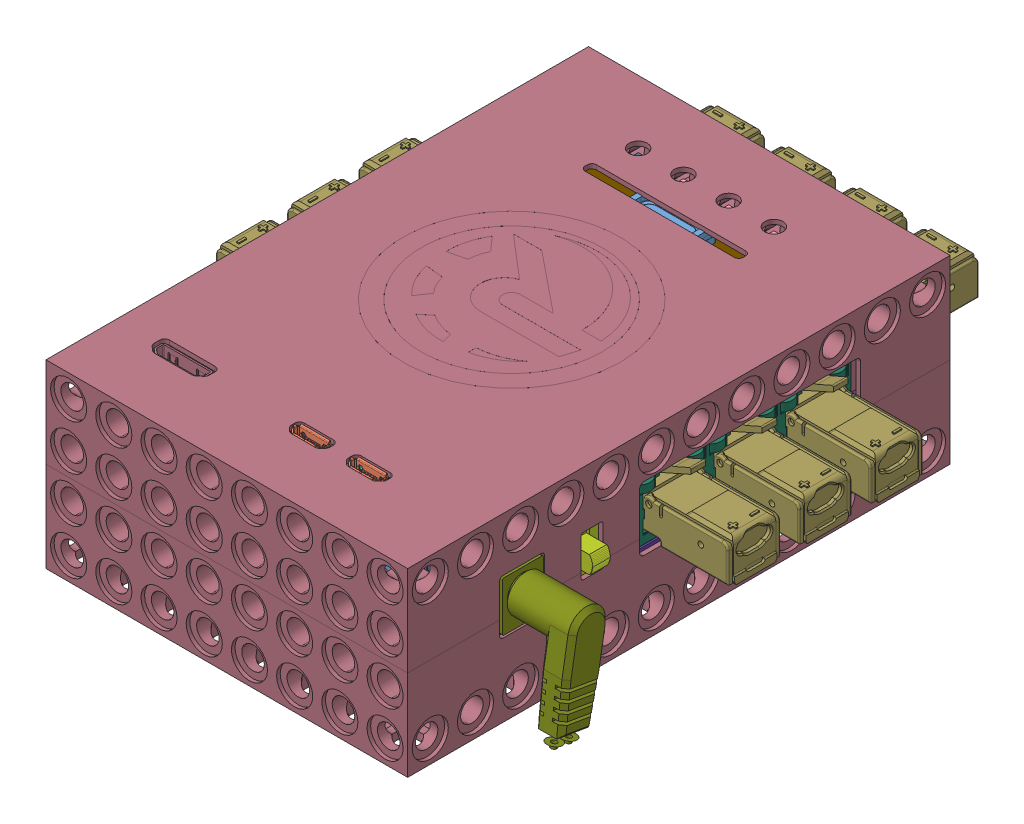
SolidWorks assembly PCBA_estimation_20190215, configuration Default. Lengths in mm. (continued)
Components (placement in the parent): (continued)
- RRRC_carrier_board-1: RRRC_carrier_board [Default] at (75.1836 8.28 47.3515) x (0 0 -1) z (0 1 0) size (102.74 81.4 21.81) (continued)
  - C112_CARRIER_3-1: C112_CARRIER_3 [Default] at origin size (0.5 1 0.5)
    - C_0402_3-1: C_0402_3 [Default] at (82 51.85 0) x (0 1 0) z (0 0 1) size (1 0.5 0.5)
  - D27_CARRIER_3-1: D27_CARRIER_3 [Default] at origin size (1.05 0.65 0.44)
    - SOD-923_3-1: SOD-923_3 [Default] at (80.75 59.9 0) x (1 0 0) z (0 -1 0) size (1.05 0.44 0.65)
  - D28_CARRIER_3-1: D28_CARRIER_3 [Default] at origin size (0.65 1.05 0.44)
    - SOD-923_3-1: SOD-923_3 [Default] at (82.05 55.6 0) x (0 1 0) z (1 0 0) size (1.05 0.44 0.65)
  - FB7_CARRIER_3-1: FB7_CARRIER_3 [Default] at origin size (0.5 1 0.5)
    - IND_0402_3-1: IND_0402_3 [Default] at (80.975 55.775 0) x (0 -1 0) z (0 0 1) size (1 0.5 0.5)
  - FB16_CARRIER_3-1: FB16_CARRIER_3 [Default] at origin size (0.5 1 0.5)
    - IND_0402_3-1: IND_0402_3 [Default] at (81 58.4 0) x (0 -1 0) z (0 0 1) size (1 0.5 0.5)
  - FU19_CARRIER_3-1: FU19_CARRIER_3 [Default] at origin size (2.3 1.5 1.25)
    - BELFUSE_0ZCK_3-1: BELFUSE_0ZCK_3 [Default] at (83.35 57.55 0) x (-1 0 0) z (0 1 0) size (2.3 1.25 1.5)
  - FU20_CARRIER_3-1: FU20_CARRIER_3 [Default] at origin size (2.3 1.5 1.25)
    - BELFUSE_0ZCK_3-1: BELFUSE_0ZCK_3 [Default] at (83.35 59.35 0) x (-1 0 0) z (0 1 0) size (2.3 1.25 1.5)
  - R100_CARRIER_3-1: R100_CARRIER_3 [Default] at origin size (1.15 0.55 0.41)
    - R_0402_3-1: R_0402_3 [Default] at (84.05 55.125 0) x (-1 0 0) z (0 1 0) size (1.15 0.41 0.55)
  - R101_CARRIER_3-1: R101_CARRIER_3 [Default] at origin size (1.15 0.55 0.41)
    - R_0402_3-1: R_0402_3 [Default] at (84.0501 54.1 0) x (-1 0 0) z (0 1 0) size (1.15 0.41 0.55)
  - R104_CARRIER_3-1: R104_CARRIER_3 [Default] at origin size (1.15 0.55 0.41)
    - R_0402_3-1: R_0402_3 [Default] at (84.0501 50.925 0) x (-1 0 0) z (0 1 0) size (1.15 0.41 0.55)
  - R141_CARRIER_3-1: R141_CARRIER_3 [Default] at origin size (1.15 0.55 0.41)
    - R_0402_3-1: R_0402_3 [Default] at (84.0501 56.125 0) x (-1 0 0) z (0 1 0) size (1.15 0.41 0.55)
  - R145_CARRIER_3-1: R145_CARRIER_3 [Default] at origin size (1.15 0.55 0.41)
    - R_0402_3-1: R_0402_3 [Default] at (84.05 52 0) x (1 0 0) z (0 -1 0) size (1.15 0.41 0.55)
  - R146_CARRIER_3-1: R146_CARRIER_3 [Default] at origin size (0.55 1.15 0.41)
    - R_0402_3-1: R_0402_3 [Default] at (81 51.85 0) x (0 1 0) z (1 0 0) size (1.15 0.41 0.55)
  - D21_CARRIER_3-1: D21_CARRIER_3 [Default] at origin size (1.05 0.65 0.44)
    - SOD-923_3-1: SOD-923_3 [Default] at (81.5 39.8 0) x (1 0 0) z (0 -1 0) size (1.05 0.44 0.65)
  - R122_CARRIER_3-1: R122_CARRIER_3 [Default] at origin size (0.55 1.15 0.41)
    - R_0402_3-1: R_0402_3 [Default] at (80.8 41.4 0) x (0 1 0) z (1 0 0) size (1.15 0.41 0.55)
  - R121_CARRIER_3-1: R121_CARRIER_3 [Default] at origin size (1.15 0.55 0.41)
    - R_0402_3-1: R_0402_3 [Default] at (84.05 41.775 0) x (1 0 0) z (0 -1 0) size (1.15 0.41 0.55)
  - R89_CARRIER_3-1: R89_CARRIER_3 [Default] at origin size (1.15 0.55 0.41)
    - R_0402_3-1: R_0402_3 [Default] at (84.05 40.725 0) x (-1 0 0) z (0 1 0) size (1.15 0.41 0.55)
  - R86_CARRIER_3-1: R86_CARRIER_3 [Default] at origin size (1.15 0.55 0.41)
    - R_0402_3-1: R_0402_3 [Default] at (84.05 42.825 0) x (-1 0 0) z (0 1 0) size (1.15 0.41 0.55)
  - R85_CARRIER_3-1: R85_CARRIER_3 [Default] at origin size (1.15 0.55 0.41)
    - R_0402_3-1: R_0402_3 [Default] at (84.05 43.825 0) x (-1 0 0) z (0 1 0) size (1.15 0.41 0.55)
  - R118_CARRIER_3-1: R118_CARRIER_3 [Default] at origin size (1.15 0.55 0.41)
    - R_0402_3-1: R_0402_3 [Default] at (84.05 44.825 0) x (-1 0 0) z (0 1 0) size (1.15 0.41 0.55)
  - FU14_CARRIER_3-1: FU14_CARRIER_3 [Default] at origin size (2.3 1.5 1.25)
    - BELFUSE_0ZCK_3-1: BELFUSE_0ZCK_3 [Default] at (83.3251 48.35 0) x (-1 0 0) z (0 1 0) size (2.3 1.25 1.5)
  - FU13_CARRIER_3-1: FU13_CARRIER_3 [Default] at origin size (2.3 1.5 1.25)
    - BELFUSE_0ZCK_3-1: BELFUSE_0ZCK_3 [Default] at (83.3251 46.5 0) x (-1 0 0) z (0 1 0) size (2.3 1.25 1.5)
  - FB10_CARRIER_3-1: FB10_CARRIER_3 [Default] at origin size (0.5 1 0.5)
    - IND_0402_3-1: IND_0402_3 [Default] at (81.025 48.475 0) x (0 1 0) z (0 0 1) size (1 0.5 0.5)
  - FB4_CARRIER_3-1: FB4_CARRIER_3 [Default] at origin size (0.5 1 0.5)
    - IND_0402_3-1: IND_0402_3 [Default] at (81 45.95 0) x (0 -1 0) z (0 0 1) size (1 0.5 0.5)
  - D19_CARRIER_3-1: D19_CARRIER_3 [Default] at origin size (0.65 1.05 0.44)
    - SOD-923_3-1: SOD-923_3 [Default] at (82 44.55 0) x (0 1 0) z (1 0 0) size (1.05 0.44 0.65)
  - D18_CARRIER_3-1: D18_CARRIER_3 [Default] at origin size (1.05 0.65 0.44)
    - SOD-923_3-1: SOD-923_3 [Default] at (81.5 50 0) x (1 0 0) z (0 -1 0) size (1.05 0.44 0.65)
  - D17_CARRIER_3-1: D17_CARRIER_3 [Default] at origin size (2 2.5 0.6)
    - 6373436816-1: 6373436816 [Default] at (76.7 41.85 0) size (2 2.5 0.6)
      - Extruded_3-1: Extruded_3 [Default] at origin size (2 2.5 0.6)
  - C101_CARRIER_3-1: C101_CARRIER_3 [Default] at origin size (0.5 1 0.5)
    - C_0402_3-1: C_0402_3 [Default] at (81.85 41.4 0) x (0 1 0) z (0 0 1) size (1 0.5 0.5)
  - C99_CARRIER_3-1: C99_CARRIER_3 [Default] at origin size (1.6 3.2 1.6)
    - C_1206_3-1: C_1206_3 [Default] at (78.35 48.05 0) x (0 1 0) z (0 0 1) size (3.2 1.6 1.6)
  - C100_CARRIER_3-1: C100_CARRIER_3 [Default] at origin size (1.6 3.2 1.6)
    - C_1206_3-1: C_1206_3 [Default] at (76.15 46.7 0) x (0 -1 0) z (0 0 1) size (3.2 1.6 1.6)
  - C72_CARRIER_3-1: C72_CARRIER_3 [Default] at origin size (0.5 1 0.5)
    - C_0402_3-1: C_0402_3 [Default] at (79.95 45.95 0) x (0 -1 0) z (0 0 1) size (1 0.5 0.5)
  - C70_CARRIER_3-1: C70_CARRIER_3 [Default] at origin size (0.5 1 0.5)
    - C_0402_3-1: C_0402_3 [Default] at (79.975 48.475 0) x (0 1 0) z (0 0 1) size (1 0.5 0.5)
  - C74_CARRIER_3-1: C74_CARRIER_3 [Default] at origin size (0.5 1 0.5)
    - C_0402_3-1: C_0402_3 [Default] at (79.95 38.3 0) x (0 1 0) z (0 0 1) size (1 0.5 0.5)
  - C76_CARRIER_3-1: C76_CARRIER_3 [Default] at origin size (0.5 1 0.5)
    - C_0402_3-1: C_0402_3 [Default] at (79.975 35.8 0) x (0 -1 0) z (0 0 1) size (1 0.5 0.5)
  - C102_CARRIER_3-1: C102_CARRIER_3 [Default] at origin size (3.2 1.6 1.6)
    - C_1206_3-1: C_1206_3 [Default] at (76.9 38.2 0) x (1 0 0) z (0 0 1) size (3.2 1.6 1.6)
  - C103_CARRIER_3-1: C103_CARRIER_3 [Default] at origin size (3.2 1.6 1.6)
    - C_1206_3-1: C_1206_3 [Default] at (76.9 35.9 0) x (1 0 0) z (0 0 1) size (3.2 1.6 1.6)
  - C105_CARRIER_3-1: C105_CARRIER_3 [Default] at origin size (0.5 1 0.5)
    - C_0402_3-1: C_0402_3 [Default] at (80.9 30.275 0) x (0 1 0) z (0 0 1) size (1 0.5 0.5)
  - D20_CARRIER_3-1: D20_CARRIER_3 [Default] at origin size (2 2.5 0.6)
    - 6373436816-1-1: 6373436816-1 [Default] at (80.7 19.55 0) size (2 2.5 0.6)
      - Extruded_3-1: Extruded_3 [Default] at origin size (2 2.5 0.6)
  - D22_CARRIER_3-1: D22_CARRIER_3 [Default] at origin size (1.05 0.65 0.44)
    - SOD-923_3-1: SOD-923_3 [Default] at (81.4 34 0) x (1 0 0) z (0 -1 0) size (1.05 0.44 0.65)
  - FB5_CARRIER_3-1: FB5_CARRIER_3 [Default] at origin size (0.5 1 0.5)
    - IND_0402_3-1: IND_0402_3 [Default] at (81.025 35.8 0) x (0 -1 0) z (0 0 1) size (1 0.5 0.5)
  - FB12_CARRIER_3-1: FB12_CARRIER_3 [Default] at origin size (0.5 1 0.5)
    - IND_0402_3-1: IND_0402_3 [Default] at (81 38.3 0) x (0 1 0) z (0 0 1) size (1 0.5 0.5)
  - FU15_CARRIER_3-1: FU15_CARRIER_3 [Default] at origin size (2.3 1.5 1.25)
    - BELFUSE_0ZCK_3-1: BELFUSE_0ZCK_3 [Default] at (83.35 35.4 0) x (-1 0 0) z (0 1 0) size (2.3 1.25 1.5)
  - FU16_CARRIER_3-1: FU16_CARRIER_3 [Default] at origin size (2.3 1.5 1.25)
    - BELFUSE_0ZCK_3-1: BELFUSE_0ZCK_3 [Default] at (83.325 38.225 0) x (-1 0 0) z (0 1 0) size (2.3 1.25 1.5)
  - R90_CARRIER_3-1: R90_CARRIER_3 [Default] at origin size (1.15 0.55 0.41)
    - R_0402_3-1: R_0402_3 [Default] at (84.075 32.875 0) x (-1 0 0) z (0 1 0) size (1.15 0.41 0.55)
  - R91_CARRIER_3-1: R91_CARRIER_3 [Default] at origin size (1.15 0.55 0.41)
    - R_0402_3-1: R_0402_3 [Default] at (84.075 31.875 0) x (-1 0 0) z (0 1 0) size (1.15 0.41 0.55)
  - R93_CARRIER_3-1: R93_CARRIER_3 [Default] at origin size (1.15 0.55 0.41)
    - R_0402_3-1: R_0402_3 [Default] at (84.075 33.875 0) x (-1 0 0) z (0 1 0) size (1.15 0.41 0.55)
  - R94_CARRIER_3-1: R94_CARRIER_3 [Default] at origin size (1.15 0.55 0.41)
    - R_0402_3-1: R_0402_3 [Default] at (84.075 29.775 0) x (-1 0 0) z (0 1 0) size (1.15 0.41 0.55)
  - R130_CARRIER_3-1: R130_CARRIER_3 [Default] at origin size (1.15 0.55 0.41)
    - R_0402_3-1: R_0402_3 [Default] at (84.075 30.825 0) x (1 0 0) z (0 -1 0) size (1.15 0.41 0.55)
  - R131_CARRIER_3-1: R131_CARRIER_3 [Default] at origin size (0.55 1.15 0.41)
    - R_0402_3-1: R_0402_3 [Default] at (81.9 30.275 0) x (0 1 0) z (1 0 0) size (1.15 0.41 0.55)
  - CON2_CARRIER_3-1: CON2_CARRIER_3 [Default] at origin size (51.17 16.61 18.92)
    - FCI_RJHSE538103-REVT1_3-1: FCI_RJHSE538103-REVT1_3 [Default] at (75.5745 0.201 0.65) x (1 0 0) z (0 -1 0) size (51.17 18.92 16.61)
  - Y1_CARRIER_3-1: Y1_CARRIER_3 [Default] at origin size (1.5 3.2 0.85)
    - TXC_9HT10_3-1: TXC_9HT10_3 [Default] at (5.75 65.75 0) x (0 -1 0) z (0 0 1) size (3.2 1.5 0.85)
  - U30_CARRIER_3-1: U30_CARRIER_3 [Default] at origin size (6.04 4.9 1.7)
    - SOIC8P127_490X604X170L60X40N_3-1: SOIC8P127_490X604X170L60X40N_3 [Default] at (27.6 30.6 0) x (1 0 0) z (0 0 1) size (6.04 4.9 1.7)
  - U29_CARRIER_3-1: U29_CARRIER_3 [Default] at origin size (14 16 2)
    - Fanstel_BT832A_3-1: Fanstel_BT832A_3 [Default] at (22.05 69 0.3) x (1 0 0) z (0 -1 0) size (14 2 16)
  - U13_CARRIER_3-1: U13_CARRIER_3 [Default] at origin size (3.1 3 0.8)
    - DFN-6(3x3)_0.45_0.95_3x3x1_HD[2,50x1,75]_3-1: DFN-6(3x3)_0.45_0.95_3x3x1_HD[2,50x1,75]_3 [Default] at (59.35 51.35 0.05) x (-1 0 0) z (0 0 1) size (3.1 3 0.8)
  - U27_CARRIER_3-1: U27_CARRIER_3 [Default] at origin size (2.03 2.13 0.6)
    - SON9P50_202X202X60L35X25T130X70_3-1: SON9P50_202X202X60L35X25T130X70_3 [Default] at (7.1 33.1 0) x (0 1 0) z (0 0 1) size (2.13 2.02 0.6)
  - U12_CARRIER_3-1: U12_CARRIER_3 [Default] at origin size (3.1 3 0.8)
    - DFN-6(3x3)_0.45_0.95_3x3x1_HD[2,50x1,75]_3-1: DFN-6(3x3)_0.45_0.95_3x3x1_HD[2,50x1,75]_3 [Default] at (54.25 51.35 0.05) x (1 0 0) z (0 0 1) size (3.1 3 0.8)
  - U25_CARRIER_3-1: U25_CARRIER_3 [Default] at origin size (4.9 6.04 1.7)
    - SOIC8P127_490X604X170L60X40N_3-1: SOIC8P127_490X604X170L60X40N_3 [Default] at (4.5 48.6 0) x (0 1 0) z (0 0 1) size (6.04 4.9 1.7)
  - U11_CARRIER_3-1: U11_CARRIER_3 [Default] at origin size (3.1 3 0.8)
    - DFN-6(3x3)_0.45_0.95_3x3x1_HD[2,50x1,75]_3-1: DFN-6(3x3)_0.45_0.95_3x3x1_HD[2,50x1,75]_3 [Default] at (46.2 51.35 0.05) x (1 0 0) z (0 0 1) size (3.1 3 0.8)
  - U10_CARRIER_3-1: U10_CARRIER_3 [Default] at origin size (4.9 6 1.5)
    - SOIC9P127_490X600X150L72X40T335X271N_3-1: SOIC9P127_490X600X150L72X40T335X271N_3 [Default] at (33.525 23.15 0) x (0 1 0) z (0 0 1) size (6 4.9 1.5)
  - U20_CARRIER_3-1: U20_CARRIER_3 [Default] at origin size (2.03 2.13 0.6)
    - SON9P50_202X202X60L35X25T130X70_3-1: SON9P50_202X202X60L35X25T130X70_3 [Default] at (7.025 58.325 0) x (0 1 0) z (0 0 1) size (2.13 2.02 0.6)
  - U18_CARRIER_3-1: U18_CARRIER_3 [Default] at origin size (3 4.9 1.1)
    - SOP10P50_300X490X110L55X22N_3-1: SOP10P50_300X490X110L55X22N_3 [Default] at (2.65 21.6 0) x (0 -1 0) z (0 0 1) size (4.9 3 1.1)
  - U3_CARRIER_3-1: U3_CARRIER_3 [Default] at origin size (3 3.1 0.8)
    - DFN-6(3x3)_0.45_0.95_3x3x1_HD[2,50x1,75]_3-1: DFN-6(3x3)_0.45_0.95_3x3x1_HD[2,50x1,75]_3 [Default] at (73.15 28.7 0.05) x (0 1 0) z (0 0 1) size (3.1 3 0.8)
  - U14_CARRIER_3-1: U14_CARRIER_3 [Default] at origin size (7.8 7.6 1.6)
    - TSSOP-24[12-12]_0.45_0.65_5.6x7.8x1.6_3-1: TSSOP-24[12-12]_0.45_0.65_5.6x7.8x1.6_3 [Default] at (65.4999 30.5001 0) x (1 0 0) z (0 0 1) size (7.8 7.6 1.6)
  - U9_CARRIER_3-1: U9_CARRIER_3 [Default] at origin size (1.8 2.1 0.5)
    - QFN12P40_170X200X50L50X20N_3-1: QFN12P40_170X200X50L50X20N_3 [Default] at (70.9 51.05 0) size (1.8 2.1 0.5)
  - U8_CARRIER_3-1: U8_CARRIER_3 [Default] at origin size (1.8 2.1 0.5)
    - QFN12P40_170X200X50L50X20N_3-1: QFN12P40_170X200X50L50X20N_3 [Default] at (70.925 37.425 0) size (1.8 2.1 0.5)
  - U7_CARRIER_3-1: U7_CARRIER_3 [Default] at origin size (1.8 2.1 0.5)
    - QFN12P40_170X200X50L50X20N_3-1: QFN12P40_170X200X50L50X20N_3 [Default] at (70.9 41.925 0) size (1.8 2.1 0.5)
  - U6_CARRIER_3-1: U6_CARRIER_3 [Default] at origin size (1.8 2.1 0.5)
    - QFN12P40_170X200X50L50X20N_3-1: QFN12P40_170X200X50L50X20N_3 [Default] at (70.85 46.475 0) x (1 0 0) z (0 0 1) size (1.8 2.1 0.5)
  - U2_CARRIER_3-1: U2_CARRIER_3 [Default] at origin size (3.1 3.1 1)
    - QFN-16[4x4]_0.30_0.50_3x3x1_HD[1.65x1.65]_3-1: QFN-16[4x4]_0.30_0.50_3x3x1_HD[1.65x1.65]_3 [Default] at (17.4 22.25 0) x (0 1 0) z (0 0 1) size (3.1 3.1 1)
  - U1_CARRIER_3-1: U1_CARRIER_3 [Default] at origin size (16 16 1.2)
    - QFP128P40_1600X1600X120L60X18N_3-1: QFP128P40_1600X1600X120L60X18N_3 [Default] at (25.15 48.025 0) x (-1 0 0) z (0 0 1) size (16 16 1.2)
  - S1_CARRIER_3-1: S1_CARRIER_3 [Default] at origin size (11.43 25.96 15.88)
    - E-SWITCH_500SDP1S1M7QEA_3-1: E-SWITCH_500SDP1S1M7QEA_3 [Default] at (25.0149 9.0198 6.4) x (0 0 -1) z (0 -1 0) size (15.88 11.43 25.96)
  - R157_CARRIER_3-1: R157_CARRIER_3 [Default] at origin size (1.15 0.55 0.41)
    - R_0402_3-1: R_0402_3 [Default] at (32.75 33.95 0) x (-1 0 0) z (0 1 0) size (1.15 0.41 0.55)
  - R156_CARRIER_3-1: R156_CARRIER_3 [Default] at origin size (0.55 1.15 0.41)
    - R_0402_3-1: R_0402_3 [Default] at (73.65 47.85 0) x (0 1 0) z (1 0 0) size (1.15 0.41 0.55)
  - R155_CARRIER_3-1: R155_CARRIER_3 [Default] at origin size (0.55 1.15 0.41)
    - R_0402_3-1: R_0402_3 [Default] at (73.65 45.8 0) x (0 -1 0) z (-1 0 0) size (1.15 0.41 0.55)
  - R154_CARRIER_3-1: R154_CARRIER_3 [Default] at origin size (0.55 1.15 0.41)
    - R_0402_3-1: R_0402_3 [Default] at (73.65 43.3 0) x (0 1 0) z (1 0 0) size (1.15 0.41 0.55)
  - R153_CARRIER_3-1: R153_CARRIER_3 [Default] at origin size (0.55 1.15 0.41)
    - R_0402_3-1: R_0402_3 [Default] at (73.65 41.3 0) x (0 -1 0) z (-1 0 0) size (1.15 0.41 0.55)
  - R152_CARRIER_3-1: R152_CARRIER_3 [Default] at origin size (0.55 1.15 0.41)
    - R_0402_3-1: R_0402_3 [Default] at (73.75 38.85 0) x (0 1 0) z (1 0 0) size (1.15 0.41 0.55)
  - R151_CARRIER_3-1: R151_CARRIER_3 [Default] at origin size (0.55 1.15 0.41)
    - R_0402_3-1: R_0402_3 [Default] at (73.75 36.85 0) x (0 -1 0) z (-1 0 0) size (1.15 0.41 0.55)
  - R150_CARRIER_3-1: R150_CARRIER_3 [Default] at origin size (0.55 1.15 0.41)
    - R_0402_3-1: R_0402_3 [Default] at (73.425 52.5 0) x (0 1 0) z (1 0 0) size (1.15 0.41 0.55)
  - R149_CARRIER_3-1: R149_CARRIER_3 [Default] at origin size (0.55 1.15 0.41)
    - R_0402_3-1: R_0402_3 [Default] at (73.425 50.5 0) x (0 -1 0) z (-1 0 0) size (1.15 0.41 0.55)
  - R148_CARRIER_3-1: R148_CARRIER_3 [Default] at origin size (0.55 1.15 0.41)
    - R_0402_3-1: R_0402_3 [Default] at (92.55 3 0) x (0 1 0) z (1 0 0) size (1.15 0.41 0.55)
  - R140_CARRIER_3-1: R140_CARRIER_3 [Default] at origin size (0.55 1.15 0.41)
    - R_0402_3-1: R_0402_3 [Default] at (90.4 74.5 0) x (0 -1 0) z (-1 0 0) size (1.15 0.41 0.55)
  - R138_CARRIER_3-1: R138_CARRIER_3 [Default] at origin size (1.15 0.55 0.41)
    - R_0402_3-1: R_0402_3 [Default] at (77.85 18.25 0) x (-1 0 0) z (0 1 0) size (1.15 0.41 0.55)
  - R137_CARRIER_3-1: R137_CARRIER_3 [Default] at origin size (1.15 0.55 0.41)
    - R_0402_3-1: R_0402_3 [Default] at (83.975 17.1 0) x (1 0 0) z (0 -1 0) size (1.15 0.41 0.55)
  - R136_CARRIER_3-1: R136_CARRIER_3 [Default] at origin size (0.55 1.15 0.41)
    - R_0402_3-1: R_0402_3 [Default] at (88.05 3 0) x (0 1 0) z (1 0 0) size (1.15 0.41 0.55)
  - R134_CARRIER_3-1: R134_CARRIER_3 [Default] at origin size (1.15 0.55 0.41)
    - R_0402_3-1: R_0402_3 [Default] at (83.975 22.25 0) x (1 0 0) z (0 -1 0) size (1.15 0.41 0.55)
  - R129_CARRIER_3-1: R129_CARRIER_3 [Default] at origin size (1.15 0.55 0.41)
    - R_0402_3-1: R_0402_3 [Default] at (84 25.15 0) x (1 0 0) z (0 -1 0) size (1.15 0.41 0.55)
  - R128_CARRIER_3-1: R128_CARRIER_3 [Default] at origin size (1.15 0.55 0.41)
    - R_0402_3-1: R_0402_3 [Default] at (84.1 36.8 0) x (1 0 0) z (0 -1 0) size (1.15 0.41 0.55)
  - R125_CARRIER_3-1: R125_CARRIER_3 [Default] at origin size (1.15 0.55 0.41)
    - R_0402_3-1: R_0402_3 [Default] at (2.85 68.3 0) x (-1 0 0) z (0 1 0) size (1.15 0.41 0.55)
  - R124_CARRIER_3-1: R124_CARRIER_3 [Default] at origin size (1.15 0.55 0.41)
    - R_0402_3-1: R_0402_3 [Default] at (2.8526 67.1098 0) x (-1 0 0) z (0 1 0) size (1.15 0.41 0.55)
  - R123_CARRIER_3-1: R123_CARRIER_3 [Default] at origin size (1.15 0.55 0.41)
    - R_0402_3-1: R_0402_3 [Default] at (4.05 17.85 0) x (1 0 0) z (0 -1 0) size (1.15 0.41 0.55)
  - R120_CARRIER_3-1: R120_CARRIER_3 [Default] at origin size (1.15 0.55 0.41)
    - R_0402_3-1: R_0402_3 [Default] at (37.5 43.05 0) x (-1 0 0) z (0 1 0) size (1.15 0.41 0.55)
  - R119_CARRIER_3-1: R119_CARRIER_3 [Default] at origin size (1.15 0.55 0.41)
    - R_0402_3-1: R_0402_3 [Default] at (84.05 39.7 0) x (1 0 0) z (0 -1 0) size (1.15 0.41 0.55)
  - R117_CARRIER_3-1: R117_CARRIER_3 [Default] at origin size (1.15 0.55 0.41)
    - R_0402_3-1: R_0402_3 [Default] at (84.05 49.85 0) x (1 0 0) z (0 -1 0) size (1.15 0.41 0.55)
  - R116_CARRIER_3-1: R116_CARRIER_3 [Default] at origin size (1.15 0.55 0.41)
    - R_0402_3-1: R_0402_3 [Default] at (37.35 47.975 0) x (1 0 0) z (0 -1 0) size (1.15 0.41 0.55)
  - R115_CARRIER_3-1: R115_CARRIER_3 [Default] at origin size (1.15 0.55 0.41)
    - R_0402_3-1: R_0402_3 [Default] at (41.65 48 0) x (1 0 0) z (0 -1 0) size (1.15 0.41 0.55)
  - R112_CARRIER_3-1: R112_CARRIER_3 [Default] at origin size (1.15 0.55 0.41)
    - R_0402_3-1: R_0402_3 [Default] at (34.55 56.7 0) x (1 0 0) z (0 -1 0) size (1.15 0.41 0.55)
  - R111_CARRIER_3-1: R111_CARRIER_3 [Default] at origin size (1.15 0.55 0.41)
    - R_0402_3-1: R_0402_3 [Default] at (34.55 55.7 0) x (1 0 0) z (0 -1 0) size (1.15 0.41 0.55)
  - R110_CARRIER_3-1: R110_CARRIER_3 [Default] at origin size (1.15 0.55 0.41)
    - R_0402_3-1: R_0402_3 [Default] at (15.3 53.175 0) x (-1 0 0) z (0 1 0) size (1.15 0.41 0.55)
  - R109_CARRIER_3-1: R109_CARRIER_3 [Default] at origin size (1.15 0.55 0.41)
    - R_0402_3-1: R_0402_3 [Default] at (15.3 54.175 0) x (-1 0 0) z (0 1 0) size (1.15 0.41 0.55)
  - R108_CARRIER_3-1: R108_CARRIER_3 [Default] at origin size (1.15 0.55 0.41)
    - R_0402_3-1: R_0402_3 [Default] at (67.575 36.825 0) x (-1 0 0) z (0 1 0) size (1.15 0.41 0.55)
  - R107_CARRIER_3-1: R107_CARRIER_3 [Default] at origin size (1.15 0.55 0.41)
    - R_0402_3-1: R_0402_3 [Default] at (67.575 37.825 0) x (-1 0 0) z (0 1 0) size (1.15 0.41 0.55)
  - R106_CARRIER_3-1: R106_CARRIER_3 [Default] at origin size (0.55 1.15 0.41)
    - R_0402_3-1: R_0402_3 [Default] at (66.9 52.55 0) x (0 1 0) z (1 0 0) size (1.15 0.41 0.55)
  - R105_CARRIER_3-1: R105_CARRIER_3 [Default] at origin size (0.55 1.15 0.41)
    - R_0402_3-1: R_0402_3 [Default] at (67.9 52.55 0) x (0 1 0) z (1 0 0) size (1.15 0.41 0.55)
  - R98_CARRIER_3-1: R98_CARRIER_3 [Default] at origin size (1.15 0.55 0.41)
    - R_0402_3-1: R_0402_3 [Default] at (83.975 21.2 0) x (-1 0 0) z (0 1 0) size (1.15 0.41 0.55)
  - R96_CARRIER_3-1: R96_CARRIER_3 [Default] at origin size (1.15 0.55 0.41)
    - R_0402_3-1: R_0402_3 [Default] at (83.975 20.2 0) x (-1 0 0) z (0 1 0) size (1.15 0.41 0.55)
  - R95_CARRIER_3-1: R95_CARRIER_3 [Default] at origin size (1.15 0.55 0.41)
    - R_0402_3-1: R_0402_3 [Default] at (83.975 19.2 0) x (-1 0 0) z (0 1 0) size (1.15 0.41 0.55)
  - R87_CARRIER_3-1: R87_CARRIER_3 [Default] at origin size (0.55 1.15 0.41)
    - R_0402_3-1: R_0402_3 [Default] at (14.95 23.325 0) x (0 -1 0) z (-1 0 0) size (1.15 0.41 0.55)
  - R84_CARRIER_3-1: R84_CARRIER_3 [Default] at origin size (1.15 0.55 0.41)
    - R_0402_3-1: R_0402_3 [Default] at (32.75 31.25 0) x (-1 0 0) z (0 1 0) size (1.15 0.41 0.55)
  - R83_CARRIER_3-1: R83_CARRIER_3 [Default] at origin size (0.55 1.15 0.41)
    - R_0402_3-1: R_0402_3 [Default] at (20.475 30.6 0) x (0 1 0) z (1 0 0) size (1.15 0.41 0.55)
  - R82_CARRIER_3-1: R82_CARRIER_3 [Default] at origin size (0.55 1.15 0.41)
    - R_0402_3-1: R_0402_3 [Default] at (17.4 26.25 0) x (0 -1 0) z (-1 0 0) size (1.15 0.41 0.55)
  - R81_CARRIER_3-1: R81_CARRIER_3 [Default] at origin size (0.55 1.15 0.41)
    - R_0402_3-1: R_0402_3 [Default] at (15.375 26.25 0) x (0 1 0) z (1 0 0) size (1.15 0.41 0.55)
  - R80_CARRIER_3-1: R80_CARRIER_3 [Default] at origin size (0.55 1.15 0.41)
    - R_0402_3-1: R_0402_3 [Default] at (21.475 30.6 0) x (0 -1 0) z (-1 0 0) size (1.15 0.41 0.55)
  - R79_CARRIER_3-1: R79_CARRIER_3 [Default] at origin size (0.55 1.15 0.41)
    - R_0402_3-1: R_0402_3 [Default] at (16.375 26.25 0) x (0 1 0) z (1 0 0) size (1.15 0.41 0.55)
  - R78_CARRIER_3-1: R78_CARRIER_3 [Default] at origin size (0.55 1.15 0.41)
    - R_0402_3-1: R_0402_3 [Default] at (23.5 30.6 0) x (0 1 0) z (1 0 0) size (1.15 0.41 0.55)
  - R77_CARRIER_3-1: R77_CARRIER_3 [Default] at origin size (1.15 0.55 0.41)
    - R_0402_3-1: R_0402_3 [Default] at (32.6 69.1 0) x (1 0 0) z (0 -1 0) size (1.15 0.41 0.55)
  - R76_CARRIER_3-1: R76_CARRIER_3 [Default] at origin size (1.15 0.55 0.41)
    - R_0402_3-1: R_0402_3 [Default] at (33.025 63.85 0) x (-1 0 0) z (0 1 0) size (1.15 0.41 0.55)
  - R75_CARRIER_3-1: R75_CARRIER_3 [Default] at origin size (0.55 1.15 0.41)
    - R_0402_3-1: R_0402_3 [Default] at (15.05 57.3 0) x (0 1 0) z (1 0 0) size (1.15 0.41 0.55)
  - R74_CARRIER_3-1: R74_CARRIER_3 [Default] at origin size (0.55 1.15 0.41)
    - R_0402_3-1: R_0402_3 [Default] at (15.05 59.45 0) x (0 1 0) z (1 0 0) size (1.15 0.41 0.55)
  - R73_CARRIER_3-1: R73_CARRIER_3 [Default] at origin size (0.55 1.15 0.41)
    - R_0402_3-1: R_0402_3 [Default] at (7.65 37.3 0) x (0 -1 0) z (-1 0 0) size (1.15 0.41 0.55)
  - R72_CARRIER_3-1: R72_CARRIER_3 [Default] at origin size (0.55 1.15 0.41)
    - R_0402_3-1: R_0402_3 [Default] at (6.65 36.8 0) x (0 1 0) z (1 0 0) size (1.15 0.41 0.55)
  - R71_CARRIER_3-1: R71_CARRIER_3 [Default] at origin size (1.15 0.55 0.41)
    - R_0402_3-1: R_0402_3 [Default] at (7.1 35.25 0) x (1 0 0) z (0 -1 0) size (1.15 0.41 0.55)
  - R70_CARRIER_3-1: R70_CARRIER_3 [Default] at origin size (0.55 1.15 0.41)
    - R_0402_3-1: R_0402_3 [Default] at (3.9 43.9 0) x (0 1 0) z (1 0 0) size (1.15 0.41 0.55)
  - R69_CARRIER_3-1: R69_CARRIER_3 [Default] at origin size (0.55 1.15 0.41)
    - R_0402_3-1: R_0402_3 [Default] at (5.15 43.9 0) x (0 1 0) z (1 0 0) size (1.15 0.41 0.55)
  - R68_CARRIER_3-1: R68_CARRIER_3 [Default] at origin size (0.55 1.15 0.41)
    - R_0402_3-1: R_0402_3 [Default] at (7.35 62.705 0) x (0 1 0) z (1 0 0) size (1.15 0.41 0.55)
  - R67_CARRIER_3-1: R67_CARRIER_3 [Default] at origin size (0.55 1.15 0.41)
    - R_0402_3-1: R_0402_3 [Default] at (40.125 27.7 0) x (0 1 0) z (1 0 0) size (1.15 0.41 0.55)
  - R66_CARRIER_3-1: R66_CARRIER_3 [Default] at origin size (0.55 1.15 0.41)
    - R_0402_3-1: R_0402_3 [Default] at (6.325 62.705 0) x (0 1 0) z (1 0 0) size (1.15 0.41 0.55)
  - R65_CARRIER_3-1: R65_CARRIER_3 [Default] at origin size (1.15 0.55 0.41)
    - R_0402_3-1: R_0402_3 [Default] at (6.75 60.625 0) x (1 0 0) z (0 -1 0) size (1.15 0.41 0.55)
  - R64_CARRIER_3-1: R64_CARRIER_3 [Default] at origin size (1.15 0.55 0.41)
    - R_0402_3-1: R_0402_3 [Default] at (2.05 17.1 0) x (1 0 0) z (0 -1 0) size (1.15 0.41 0.55)
  - R63_CARRIER_3-1: R63_CARRIER_3 [Default] at origin size (0.55 1.15 0.41)
    - R_0402_3-1: R_0402_3 [Default] at (1.2 26.3 0) x (0 -1 0) z (-1 0 0) size (1.15 0.41 0.55)
  - R62_CARRIER_3-1: R62_CARRIER_3 [Default] at origin size (1.15 0.55 0.41)
    - R_0402_3-1: R_0402_3 [Default] at (5.425 26.65 0) x (-1 0 0) z (0 1 0) size (1.15 0.41 0.55)
  - R61_CARRIER_3-1: R61_CARRIER_3 [Default] at origin size (0.55 1.15 0.41)
    - R_0402_3-1: R_0402_3 [Default] at (39.075 27.7 0) x (0 -1 0) z (-1 0 0) size (1.15 0.41 0.55)
  - R60_CARRIER_3-1: R60_CARRIER_3 [Default] at origin size (0.55 1.15 0.41)
    - R_0402_3-1: R_0402_3 [Default] at (2.175 26.3 0) x (0 -1 0) z (-1 0 0) size (1.15 0.41 0.55)
  - R59_CARRIER_3-1: R59_CARRIER_3 [Default] at origin size (0.55 1.15 0.41)
    - R_0402_3-1: R_0402_3 [Default] at (3.175 26.3 0) x (0 -1 0) z (-1 0 0) size (1.15 0.41 0.55)
  - R58_CARRIER_3-1: R58_CARRIER_3 [Default] at origin size (0.55 1.15 0.41)
    - R_0402_3-1: R_0402_3 [Default] at (43.55 33.875 0) x (0 1 0) z (1 0 0) size (1.15 0.41 0.55)
  - R57_CARRIER_3-1: R57_CARRIER_3 [Default] at origin size (0.55 1.15 0.41)
    - R_0402_3-1: R_0402_3 [Default] at (44.625 33.875 0) x (0 -1 0) z (-1 0 0) size (1.15 0.41 0.55)
  - R56_CARRIER_3-1: R56_CARRIER_3 [Default] at origin size (1.15 0.55 0.41)
    - R_0402_3-1: R_0402_3 [Default] at (73.3 54.6 0) x (-1 0 0) z (0 1 0) size (1.15 0.41 0.55)
  - R55_CARRIER_3-1: R55_CARRIER_3 [Default] at origin size (0.55 1.15 0.41)
    - R_0402_3-1: R_0402_3 [Default] at (67.4 59.125 0) x (0 1 0) z (1 0 0) size (1.15 0.41 0.55)
  - R54_CARRIER_3-1: R54_CARRIER_3 [Default] at origin size (1.15 0.55 0.41)
    - R_0402_3-1: R_0402_3 [Default] at (62.5 59.75 0) x (1 0 0) z (0 -1 0) size (1.15 0.41 0.55)
  - R53_CARRIER_3-1: R53_CARRIER_3 [Default] at origin size (0.55 1.15 0.41)
    - R_0402_3-1: R_0402_3 [Default] at (6.95 43.9 0) x (0 -1 0) z (-1 0 0) size (1.15 0.41 0.55)
  - R52_CARRIER_3-1: R52_CARRIER_3 [Default] at origin size (1.15 0.55 0.41)
    - R_0402_3-1: R_0402_3 [Default] at (62.45 56.7 0) x (1 0 0) z (0 -1 0) size (1.15 0.41 0.55)
  - R51_CARRIER_3-1: R51_CARRIER_3 [Default] at origin size (1.15 0.55 0.41)
    - R_0402_3-1: R_0402_3 [Default] at (66.925 55.55 0) x (-1 0 0) z (0 1 0) size (1.15 0.41 0.55)
  - R50_CARRIER_3-1: R50_CARRIER_3 [Default] at origin size (1.15 0.55 0.41)
    - R_0402_3-1: R_0402_3 [Default] at (71.3 54.6 0) x (1 0 0) z (0 -1 0) size (1.15 0.41 0.55)
  - R49_CARRIER_3-1: R49_CARRIER_3 [Default] at origin size (0.55 1.15 0.41)
    - R_0402_3-1: R_0402_3 [Default] at (87.6 74.5 0) x (0 -1 0) z (-1 0 0) size (1.15 0.41 0.55)
  - R45_CARRIER_3-1: R45_CARRIER_3 [Default] at origin size (1.15 0.55 0.41)
    - R_0402_3-1: R_0402_3 [Default] at (73.4 59.65 0) x (1 0 0) z (0 -1 0) size (1.15 0.41 0.55)
  - R41_CARRIER_3-1: R41_CARRIER_3 [Default] at origin size (0.55 1.15 0.41)
    - R_0402_3-1: R_0402_3 [Default] at (68.4 59.125 0) x (0 1 0) z (1 0 0) size (1.15 0.41 0.55)
  - R27_CARRIER_3-1: R27_CARRIER_3 [Default] at origin size (0.55 1.15 0.41)
    - R_0402_3-1: R_0402_3 [Default] at (31.975 7.8 0) x (0 1 0) z (1 0 0) size (1.15 0.41 0.55)
  - R23_CARRIER_3-1: R23_CARRIER_3 [Default] at origin size (1.15 0.55 0.41)
    - R_0402_3-1: R_0402_3 [Default] at (38.615 17.3501 0) x (-1 0 0) z (0 1 0) size (1.15 0.41 0.55)
  - R19_CARRIER_3-1: R19_CARRIER_3 [Default] at origin size (0.55 1.15 0.41)
    - R_0402_3-1: R_0402_3 [Default] at (50.25 17.9 0) x (0 -1 0) z (-1 0 0) size (1.15 0.41 0.55)
  - R14_CARRIER_3-1: R14_CARRIER_3 [Default] at origin size (1.15 0.55 0.41)
    - R_0402_3-1: R_0402_3 [Default] at (67.75 22.65 0) x (-1 0 0) z (0 1 0) size (1.15 0.41 0.55)
  - R13_CARRIER_3-1: R13_CARRIER_3 [Default] at origin size (1.15 0.55 0.41)
    - R_0402_3-1: R_0402_3 [Default] at (69.4 17.45 0) x (1 0 0) z (0 -1 0) size (1.15 0.41 0.55)
  - R12_CARRIER_3-1: R12_CARRIER_3 [Default] at origin size (1.15 0.55 0.41)
    - R_0402_3-1: R_0402_3 [Default] at (73.45 17.45 0) x (1 0 0) z (0 -1 0) size (1.15 0.41 0.55)
  - R10_CARRIER_3-1: R10_CARRIER_3 [Default] at origin size (0.55 1.15 0.41)
    - R_0402_3-1: R_0402_3 [Default] at (72.875 21.125 0) x (0 1 0) z (1 0 0) size (1.15 0.41 0.55)
  - R9_CARRIER_3-1: R9_CARRIER_3 [Default] at origin size (0.55 1.15 0.41)
    - R_0402_3-1: R_0402_3 [Default] at (68.825 21.125 0) x (0 1 0) z (1 0 0) size (1.15 0.41 0.55)
  - R8_CARRIER_3-1: R8_CARRIER_3 [Default] at origin size (1.15 0.55 0.41)
    - R_0402_3-1: R_0402_3 [Default] at (65.75 22.65 0) x (1 0 0) z (0 -1 0) size (1.15 0.41 0.55)
  - R7_CARRIER_3-1: R7_CARRIER_3 [Default] at origin size (1.15 0.55 0.41)
    - R_0402_3-1: R_0402_3 [Default] at (67.275 17.525 0) x (1 0 0) z (0 -1 0) size (1.15 0.41 0.55)
  - R6_CARRIER_3-1: R6_CARRIER_3 [Default] at origin size (1.15 0.55 0.41)
    - R_0402_3-1: R_0402_3 [Default] at (77.85 17.1 0) x (1 0 0) z (0 -1 0) size (1.15 0.41 0.55)
  - R5_CARRIER_3-1: R5_CARRIER_3 [Default] at origin size (0.55 1.15 0.41)
    - R_0402_3-1: R_0402_3 [Default] at (22.95 33.55 0) x (0 -1 0) z (-1 0 0) size (1.15 0.41 0.55)
  - R4_CARRIER_3-1: R4_CARRIER_3 [Default] at origin size (1.15 0.55 0.41)
    - R_0402_3-1: R_0402_3 [Default] at (24.15 38.15 0) x (1 0 0) z (0 -1 0) size (1.15 0.41 0.55)
  - R3_CARRIER_3-1: R3_CARRIER_3 [Default] at origin size (1.15 0.55 0.41)
    - R_0402_3-1: R_0402_3 [Default] at (29.9 33.95 0) x (-1 0 0) z (0 1 0) size (1.15 0.41 0.55)
  - R2_CARRIER_3-1: R2_CARRIER_3 [Default] at origin size (0.55 1.15 0.41)
    - R_0402_3-1: R_0402_3 [Default] at (19.675 58.225 0) x (0 1 0) z (1 0 0) size (1.15 0.41 0.55)
  - R1_CARRIER_3-1: R1_CARRIER_3 [Default] at origin size (0.55 1.15 0.41)
    - R_0402_3-1: R_0402_3 [Default] at (20.875 58.225 0) x (0 1 0) z (1 0 0) size (1.15 0.41 0.55)
  - Q12_CARRIER_3-1: Q12_CARRIER_3 [Default] at origin size (3.05 3 1.41)
    - SOT95P255X140-3N_3-1: SOT95P255X140-3N_3 [Default] at (36.825 45.475 0) x (0 1 0) z (0 0 1) size (3 3.05 1.41)
  - Q11_CARRIER_3-1: Q11_CARRIER_3 [Default] at origin size (3.05 3 1.41)
    - SOT95P255X140-3N_3-1: SOT95P255X140-3N_3 [Default] at (42.65 45.525 0) x (0 1 0) z (0 0 1) size (3 3.05 1.41)
  - Q10_CARRIER_3-1: Q10_CARRIER_3 [Default] at origin size (3.05 3 1.41)
    - SOT95P255X140-3N_3-1: SOT95P255X140-3N_3 [Default] at (32.2 66.525 0) x (0 -1 0) z (0 0 1) size (3 3.05 1.41)
  - Q9_CARRIER_3-1: Q9_CARRIER_3 [Default] at origin size (1.2 1.2 0.55)
    - SOT-723_3-1: SOT-723_3 [Default] at (5.325 25.2 0) x (-1 0 0) z (0 0 1) size (1.2 1.2 0.55)
  - Q8_CARRIER_3-1: Q8_CARRIER_3 [Default] at origin size (3 3.05 1.41)
    - SOT95P255X140-3N_3-1: SOT95P255X140-3N_3 [Default] at (12 15.5 0) x (1 0 0) z (0 0 1) size (3 3.05 1.41)
  - Q7_CARRIER_3-1: Q7_CARRIER_3 [Default] at origin size (3.05 3 1.41)
    - SOT95P255X140-3N_3-1: SOT95P255X140-3N_3 [Default] at (72.6 57.1 0) x (0 1 0) z (0 0 1) size (3 3.05 1.41)
  - Q2_CARRIER_3-1: Q2_CARRIER_3 [Default] at origin size (3.05 3 1.41)
    - SOT95P255X140-3N_3-1: SOT95P255X140-3N_3 [Default] at (66.45 20.2 0) x (0 -1 0) z (0 0 1) size (3 3.05 1.41)
  - Q1_CARRIER_3-1: Q1_CARRIER_3 [Default] at origin size (3.05 3 1.41)
    - SOT95P255X140-3N_3-1: SOT95P255X140-3N_3 [Default] at (20.65 34.4 0) x (0 1 0) z (0 0 1) size (3 3.05 1.41)
  - L3_CARRIER_3-1: L3_CARRIER_3 [Default] at origin size (5.18 5.49 2)
    - Vishay_2020BZ-01_3-1: Vishay_2020BZ-01_3 [Default] at (3.2 30.95 0) x (0 1 0) z (1 0 0) size (5.49 2 5.18)
  - L2_CARRIER_3-1: L2_CARRIER_3 [Default] at origin size (5.18 5.49 2)
    - Vishay_2020BZ-01_3-1: Vishay_2020BZ-01_3 [Default] at (3.075 56.325 0) x (0 1 0) z (1 0 0) size (5.49 2 5.18)
  - L1_CARRIER_3-1: L1_CARRIER_3 [Default] at origin size (3.22 2.52 1.72)
    - Taiyo_BRL3225_3-1: Taiyo_BRL3225_3 [Default] at (26.2 34.95 0.01) x (-1 0 0) z (0 1 0) size (3.22 1.72 2.52)
  - FU18_CARRIER_3-1: FU18_CARRIER_3 [Default] at origin size (2.3 1.5 1.25)
    - BELFUSE_0ZCK_3-1: BELFUSE_0ZCK_3 [Default] at (83.25 26.55 0) x (-1 0 0) z (0 1 0) size (2.3 1.25 1.5)
  - FU17_CARRIER_3-1: FU17_CARRIER_3 [Default] at origin size (2.3 1.5 1.25)
    - BELFUSE_0ZCK_3-1: BELFUSE_0ZCK_3 [Default] at (83.225 23.7 0) x (-1 0 0) z (0 1 0) size (2.3 1.25 1.5)
  - FU12_CARRIER_3-1: FU12_CARRIER_3 [Default] at origin size (1.5 2.3 1.25)
    - BELFUSE_0ZCK_3-1: BELFUSE_0ZCK_3 [Default] at (69.875 58.4 0) x (0 1 0) z (1 0 0) size (2.3 1.25 1.5)
  - FU11_CARRIER_3-1: FU11_CARRIER_3 [Default] at origin size (1.5 2.3 1.25)
    - BELFUSE_0ZCK_3-1: BELFUSE_0ZCK_3 [Default] at (64.4 58.45 0) x (0 1 0) z (1 0 0) size (2.3 1.25 1.5)
  - FU2_CARRIER_3-1: FU2_CARRIER_3 [Default] at origin size (1.5 2.3 1.25)
    - BELFUSE_0ZCK_3-1: BELFUSE_0ZCK_3 [Default] at (71.375 19.075 0) x (0 -1 0) z (-1 0 0) size (2.3 1.25 1.5)
  - FU1_CARRIER_3-1: FU1_CARRIER_3 [Default] at origin size (1.5 2.3 1.25)
    - BELFUSE_0ZCK_3-1: BELFUSE_0ZCK_3 [Default] at (75.6 18.6 0) x (0 -1 0) z (-1 0 0) size (2.3 1.25 1.5)
  - FB14_CARRIER_3-1: FB14_CARRIER_3 [Default] at origin size (0.5 1 0.5)
    - IND_0402_3-1: IND_0402_3 [Default] at (80.9 25.425 0) x (0 1 0) z (0 0 1) size (1 0.5 0.5)
  - FB6_CARRIER_3-1: FB6_CARRIER_3 [Default] at origin size (0.5 1 0.5)
    - IND_0402_3-1: IND_0402_3 [Default] at (80.925 22.925 0) x (0 -1 0) z (0 0 1) size (1 0.5 0.5)
  - FB3_CARRIER_3-1: FB3_CARRIER_3 [Default] at origin size (0.5 1 0.5)
    - IND_0402_3-1: IND_0402_3 [Default] at (17.05 7.85 0) x (0 -1 0) z (0 0 1) size (1 0.5 0.5)
  - FB2_CARRIER_3-1: FB2_CARRIER_3 [Default] at origin size (0.8 1.6 0.8)
    - IND_0603_3-1: IND_0603_3 [Default] at (36.5 54.525 0) x (0 -1 0) z (0 0 1) size (1.6 0.8 0.8)
  - FB1_CARRIER_3-1: FB1_CARRIER_3 [Default] at origin size (0.8 1.6 0.8)
    - IND_0603_3-1: IND_0603_3 [Default] at (34.95 58.975 0) x (0 -1 0) z (0 0 1) size (1.6 0.8 0.8)
  - D49_CARRIER_3-1: D49_CARRIER_3 [Default] at origin size (1.6 3.6 1.3)
    - SOD360X160X130L37X85N_3-1: SOD360X160X130L37X85N_3 [Default] at (39.75 45.475 0) x (0 1 0) z (0 0 1) size (3.6 1.6 1.3)
  - D48_CARRIER_3-1: D48_CARRIER_3 [Default] at origin size (1.6 3.6 1.3)
    - SOD360X160X130L37X85N_3-1: SOD360X160X130L37X85N_3 [Default] at (45.55 45.525 0) x (0 1 0) z (0 0 1) size (3.6 1.6 1.3)
  - D47_CARRIER_3-1: D47_CARRIER_3 [Default] at origin size (0.55 1.15 0.41)
    - R_0402_3-1: R_0402_3 [Default] at (8.2 15.05 0) x (0 -1 0) z (-1 0 0) size (1.15 0.41 0.55)
  - D46_CARRIER_3-1: D46_CARRIER_3 [Default] at origin size (1.05 0.65 0.44)
    - SOD-923_3-1: SOD-923_3 [Default] at (63.9 55.6 0) x (1 0 0) z (0 -1 0) size (1.05 0.44 0.65)
  - D45_CARRIER_3-1: D45_CARRIER_3 [Default] at origin size (1.05 0.65 0.44)
    - SOD-923_3-1: SOD-923_3 [Default] at (69.2 56.05 0) x (1 0 0) z (0 -1 0) size (1.05 0.44 0.65)
  - D44_CARRIER_3-1: D44_CARRIER_3 [Default] at origin size (1.05 0.65 0.44)
    - SOD-923_3-1: SOD-923_3 [Default] at (71.6 59.65 0) x (1 0 0) z (0 -1 0) size (1.05 0.44 0.65)
  - D30_CARRIER_3-1: D30_CARRIER_3 [Default] at origin size (1.05 0.65 0.44)
    - SOD-923_3-1: SOD-923_3 [Default] at (31.9 16.1 0) x (-1 0 0) z (0 1 0) size (1.05 0.44 0.65)
  - D29_CARRIER_3-1: D29_CARRIER_3 [Default] at origin size (1.05 0.65 0.44)
    - SOD-923_3-1: SOD-923_3 [Default] at (16.425 16.1 0) x (1 0 0) z (0 -1 0) size (1.05 0.44 0.65)
  - D25_CARRIER_3-1: D25_CARRIER_3 [Default] at origin size (0.65 1.05 0.44)
    - SOD-923_3-1: SOD-923_3 [Default] at (81.95 21.95 0) x (0 1 0) z (1 0 0) size (1.05 0.44 0.65)
  - D23_CARRIER_3-1: D23_CARRIER_3 [Default] at origin size (2 2.5 0.6)
    - 6373436816-2-1: 6373436816-2 [Default] at (76.575 52.975 0) size (2 2.5 0.6)
      - Extruded_3-1: Extruded_3 [Default] at origin size (2 2.5 0.6)
  - D16_CARRIER_3-1: D16_CARRIER_3 [Default] at origin size (6.5 4 1.11)
    - Diodes_PowerDI5_3-1: Diodes_PowerDI5_3 [Default] at (4.35 40.4 0.05) x (0 1 0) z (1 0 0) size (4 1.11 6.5)
  - D7_CARRIER_3-1: D7_CARRIER_3 [Default] at origin size (1.15 0.55 0.41)
    - R_0402_3-1: R_0402_3 [Default] at (64.475 25.4 0) x (-1 0 0) z (0 1 0) size (1.15 0.41 0.55)
  - D6_CARRIER_3-1: D6_CARRIER_3 [Default] at origin size (1.15 0.55 0.41)
    - R_0402_3-1: R_0402_3 [Default] at (62.475 25.4 0) x (1 0 0) z (0 -1 0) size (1.15 0.41 0.55)
  - D5_CARRIER_3-1: D5_CARRIER_3 [Default] at origin size (1.05 0.65 0.44)
    - SOD-923_3-1: SOD-923_3 [Default] at (65.35 17.55 0) x (1 0 0) z (0 -1 0) size (1.05 0.44 0.65)
  - D4_CARRIER_3-1: D4_CARRIER_3 [Default] at origin size (1.15 0.55 0.41)
    - R_0402_3-1: R_0402_3 [Default] at (66.55 25.4 0) x (1 0 0) z (0 -1 0) size (1.15 0.41 0.55)
  - D3_CARRIER_3-1: D3_CARRIER_3 [Default] at origin size (1.15 0.55 0.41)
    - R_0402_3-1: R_0402_3 [Default] at (68.55 25.4 0) x (-1 0 0) z (0 1 0) size (1.15 0.41 0.55)
  - D2_CARRIER_3-1: D2_CARRIER_3 [Default] at origin size (1.05 0.65 0.44)
    - SOD-923_3-1: SOD-923_3 [Default] at (70.8 21.45 0) x (1 0 0) z (0 -1 0) size (1.05 0.44 0.65)
